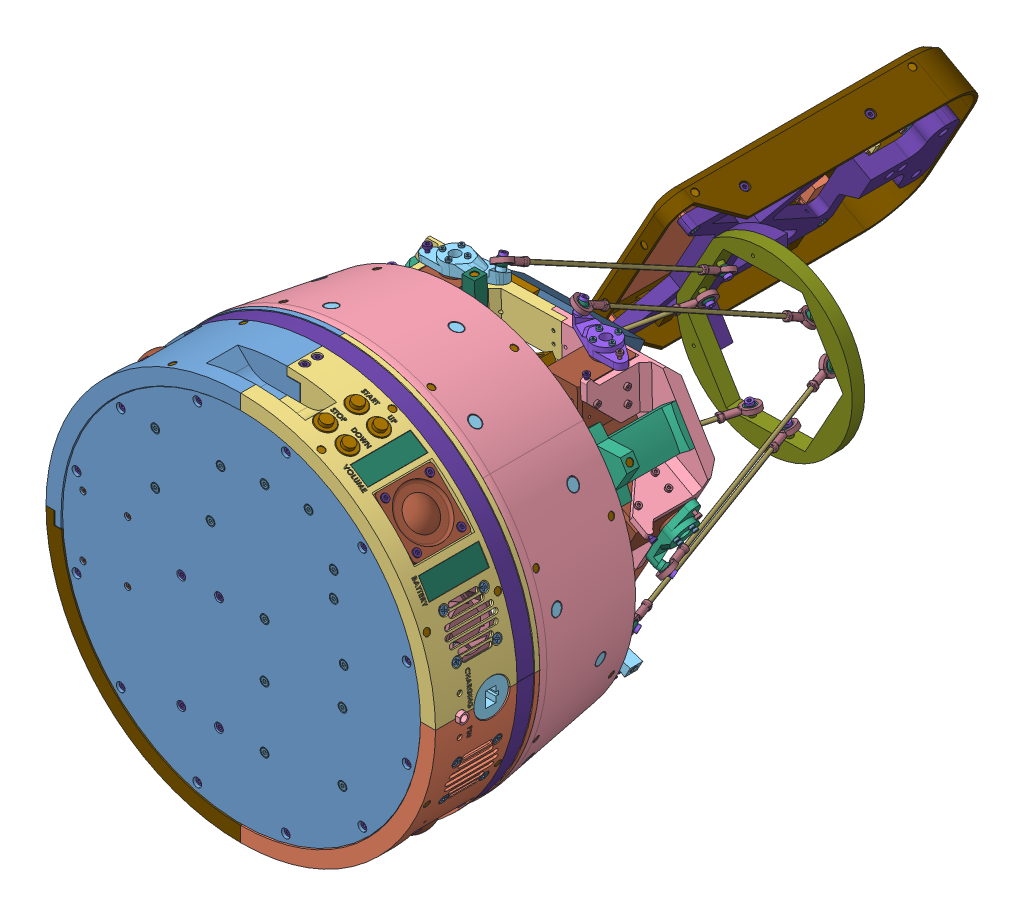
SolidWorks assembly robot xavier, configuration Défaut. Lengths in mm. (continued)
Components (placement in the parent): (continued)
- stewart-1: stewart [Défaut] at (-100.6475 26.8239 383.3519) x (-0.481912 -0.876219 0) z (0 0 1) size (270.43 245.67 405.82) (continued)
  - stewart bottom-1: stewart bottom [Défaut] at (51.9082 27.1683 257.1781) size (269.04 236.07 88.26) (flexible) (continued)
    - M2.5x8mm plastic-44: M2.5x8mm plastic [Défaut] at (-155.432 88.9962 153.3057) x (-0.891812 0 -0.452406) z (0 1 0) size (4.5 4.5 9.9)
    - M2.5x8mm plastic-45: M2.5x8mm plastic [Défaut] at (-0.6388 88.9962 153.514) x (0.993528 0 0.11359) z (0 1 0) size (4.5 4.5 9.9)
    - M2.5x8mm plastic-46: M2.5x8mm plastic [Défaut] at (43.8302 11.9975 156.9587) x (-0.496387 -0.859767 0.120004) z (0.866025 -0.5 0) size (4.5 4.5 9.9)
    - M3x8mm plastic-8: M3x8mm plastic [Défaut] at (-150.8412 50.5806 138.5562) x (0.25 0.433013 -0.866025) z (0.866025 -0.5 0) size (5.5 5.5 10.3)
    - M3x8mm plastic-9: M3x8mm plastic [Défaut] at (-164.3412 27.1979 138.5562) x (0.25 0.433013 -0.866025) z (0.866025 -0.5 0) size (5.5 5.5 10.3)
  - stewart rod-1: stewart rod [Défaut] at (34.7387 42.7785 243.5766) x (0.831609 0.550333 -0.074565) z (0.269993 -0.283304 0.920241) size (3 3 170)
  - stewart rod-2: stewart rod [Défaut] at (1.3025 -15.1346 243.6154) x (0.750903 0.658079 -0.055466) z (0.288475 -0.251293 0.923923) size (3 3 170)
  - stewart rod-3: stewart rod [Défaut] at (-69.2882 42.8434 243.2148) x (-0.526243 -0.723245 -0.447198) z (-0.37195 -0.277144 0.885914) size (3 3 170)
  - stewart rod-4: stewart rod [Défaut] at (-35.7774 -15.199 243.2264) x (0.751318 -0.64548 0.137392) z (-0.383348 -0.257403 0.887011) size (3 3 170)
  - stewart rod-5: stewart rod [Défaut] at (-50.6979 74.9201 243.922) x (-0.993577 0.094375 -0.062435) z (-0.031266 0.301309 0.953014) size (3 3 170)
  - stewart rod-6: stewart rod [Défaut] at (16.1837 74.9201 243.9023) x (0.359224 -0.882055 0.304856) z (-0.067343 0.301309 0.951145) size (3 3 170)
  - ball joint-1: ball joint [Défaut] at (86.3791 -15.0497 429.378) x (-0.641299 -0.765812 -0.047608) z (-0.269993 0.283304 -0.920241) size (14 8.06 27.54) (flexible)
    - ball joint body-1: ball joint body [Défaut] at (-2.323 -1.7007 27.3075) size (14 5.52 27.54)
    - ball joint liner-1: ball joint liner [Défaut] at (-2.323 -1.7007 20.7692) x (0.998229 0 -0.059488) z (0.059488 0 0.998229) size (9 3.5 9)
    - ball joint ball-1: ball joint ball [Défaut] at (-2.323 -1.7007 20.7692) x (-0.872539 0.157807 0.462355) z (-0.455394 0.079955 -0.886692) size (8 6 8)
  - ball joint-2: ball joint [Défaut] at (56.6193 -65.8542 430.4324) x (-0.789576 -0.608272 0.081087) z (-0.288475 0.251293 -0.923923) size (14 8.06 27.54) (flexible)
    - ball joint body-1: ball joint body [Défaut] at (-2.323 -1.7007 27.3075) size (14 5.52 27.54)
    - ball joint liner-1: ball joint liner [Défaut] at (-2.323 -1.7007 20.7692) x (0.94632 0 -0.323231) z (0.323231 0 0.94632) size (9 3.5 9)
    - ball joint ball-1: ball joint ball [Défaut] at (-2.323 -1.7007 20.7692) x (0.587551 -0.223397 -0.777738) z (0.725979 -0.278987 0.628586) size (8 6 8)
  - ball joint-3: ball joint [Défaut] at (-142.8187 -10.735 422.8134) x (-0.09653 0.960763 0.260032) z (0.37195 0.277144 -0.885914) size (14 8.06 27.54) (flexible)
    - ball joint body-1: ball joint body [Défaut] at (-2.323 -1.7007 27.3075) size (14 5.52 27.54)
    - ball joint liner-1: ball joint liner [Défaut] at (-2.323 -1.7007 20.7692) x (-0.616395 0 -0.787437) z (0.787437 0 -0.616395) size (9 3.5 9)
    - ball joint ball-1: ball joint ball [Défaut] at (-2.323 -1.7007 20.7692) x (0.165408 0.04529 -0.985185) z (0.919478 -0.368332 0.137444) size (8 6 8)
  - ball joint-4: ball joint [Défaut] at (-114.0751 -64.3814 422.0659) x (-0.810009 0.555134 -0.188975) z (0.383348 0.257403 -0.887011) size (14 8.06 27.54) (flexible)
    - ball joint body-1: ball joint body [Défaut] at (-2.323 -1.7007 27.3075) size (14 5.52 27.54)
    - ball joint liner-1: ball joint liner [Défaut] at (-2.323 -1.7007 20.7692) x (-0.982349 0 0.18706) z (-0.18706 0 -0.982349) size (9 3.5 9)
    - ball joint ball-1: ball joint ball [Défaut] at (-2.323 -1.7007 20.7692) x (0.172931 0.183122 -0.967761) z (0.917508 0.327341 0.225891) size (8 6 8)
  - ball joint-5: ball joint [Défaut] at (-0.0745 136.4534 434.9058) x (-0.957396 -0.287828 0.023394) z (0.067343 -0.301309 -0.951145) size (14 8.06 27.54) (flexible)
    - ball joint body-1: ball joint body [Défaut] at (-2.323 -1.7007 27.3075) size (14 5.52 27.54)
    - ball joint liner-1: ball joint liner [Défaut] at (-2.323 -1.7007 20.7692) x (-0.714828 0 0.6993) z (-0.6993 0 -0.714828) size (9 3.5 9)
    - ball joint ball-1: ball joint ball [Défaut] at (-2.323 -1.7007 20.7692) x (0.92076 0.200492 0.334671) z (-0.308893 -0.149333 0.9393) size (8 6 8)
  - ball joint-6: ball joint [Défaut] at (-58.7526 137.7306 435.0318) x (-0.960472 0.25482 -0.112076) z (0.031266 -0.301309 -0.953014) size (14 8.06 27.54) (flexible)
    - ball joint body-1: ball joint body [Défaut] at (-2.323 -1.7007 27.3075) size (14 5.52 27.54)
    - ball joint liner-1: ball joint liner [Défaut] at (-2.323 -1.7007 20.7692) x (-0.066426 0 0.997791) z (-0.997791 0 -0.066426) size (9 3.5 9)
    - ball joint ball-1: ball joint ball [Défaut] at (-2.323 -1.7007 20.7692) x (0.463327 -0.040267 -0.885272) z (0.854034 -0.246363 0.458183) size (8 6 8)
  - ball joint-7: ball joint [Défaut] at (28.9713 51.1868 213.8362) x (0.611438 -0.687853 -0.391154) z (0.269993 -0.283304 0.920241) size (14 8.06 27.54) (flexible)
    - ball joint body-1: ball joint body [Défaut] at (-2.323 -1.7007 27.3075) size (14 5.52 27.54)
    - ball joint liner-1: ball joint liner [Défaut] at (-2.323 -1.7007 20.7692) x (0.810022 0 0.5864) z (-0.5864 0 0.810022) size (9 3.5 9)
    - ball joint ball-1: ball joint ball [Défaut] at (-2.323 -1.7007 20.7692) x (-0.955028 0.27367 0.114134) z (-0.137201 -0.066622 -0.9883) size (8 6 8)
  - ball joint-8: ball joint [Défaut] at (21.1642 65.5917 214.2944) x (0.814856 -0.533495 0.226697) z (-0.067343 0.301309 0.951145) size (14 8.06 27.54) (flexible)
    - ball joint body-1: ball joint body [Défaut] at (-2.323 -1.7007 27.3075) size (14 5.52 27.54)
    - ball joint liner-1: ball joint liner [Défaut] at (-2.323 -1.7007 20.7692) x (0.990267 0 0.139182) z (-0.139182 0 0.990267) size (9 3.5 9)
    - ball joint ball-1: ball joint ball [Défaut] at (-2.323 -1.7007 20.7692) x (-0.414294 0.066271 -0.907727) z (0.825998 -0.391457 -0.405572) size (8 6 8)
  - ball joint-9: ball joint [Défaut] at (-59.2368 53.9166 215.5598) x (-0.006343 0.955126 0.296133) z (-0.37195 -0.277144 0.885914) size (14 8.06 27.54) (flexible)
    - ball joint body-1: ball joint body [Défaut] at (-2.323 -1.7007 27.3075) size (14 5.52 27.54)
    - ball joint liner-1: ball joint liner [Défaut] at (-2.323 -1.7007 20.7692) x (0.770033 0 -0.638005) z (0.638005 0 0.770033) size (9 3.5 9)
    - ball joint ball-1: ball joint ball [Défaut] at (-2.323 -1.7007 20.7692) x (-0.855754 0.383962 -0.346783) z (0.314359 -0.146489 -0.937934) size (8 6 8)
  - ball joint-10: ball joint [Défaut] at (-49.6158 68.2312 213.2212) x (0.619017 0.754451 -0.218223) z (-0.031266 0.301309 0.953014) size (14 8.06 27.54) (flexible)
    - ball joint body-1: ball joint body [Défaut] at (-2.323 -1.7007 27.3075) size (14 5.52 27.54)
    - ball joint liner-1: ball joint liner [Défaut] at (-2.323 -1.7007 20.7692) x (0.987977 0 -0.154599) z (0.154599 0 0.987977) size (9 3.5 9)
    - ball joint ball-1: ball joint ball [Défaut] at (-2.323 -1.7007 20.7692) x (-0.498287 -0.076288 -0.863649) z (0.860004 0.08291 -0.503507) size (8 6 8)
  - ball joint-11: ball joint [Défaut] at (-21.1891 -6.7985 216.6734) x (0.851424 -0.47068 0.231381) z (-0.383348 -0.257403 0.887011) size (14 8.06 27.54) (flexible)
    - ball joint body-1: ball joint body [Défaut] at (-2.323 -1.7007 27.3075) size (14 5.52 27.54)
    - ball joint liner-1: ball joint liner [Défaut] at (-2.323 -1.7007 20.7692) x (0.919675 0 -0.39268) z (0.39268 0 0.919675) size (9 3.5 9)
    - ball joint ball-1: ball joint ball [Défaut] at (-2.323 -1.7007 20.7692) x (-0.561763 -0.31173 -0.76632) z (0.717246 0.278105 -0.638918) size (8 6 8)
  - ball joint-12: ball joint [Défaut] at (-5.5073 -5.4469 214.4911) x (0.957486 0.077261 -0.27794) z (0.288475 -0.251293 0.923923) size (14 8.06 27.54) (flexible)
    - ball joint body-1: ball joint body [Défaut] at (-2.323 -1.7007 27.3075) size (14 5.52 27.54)
    - ball joint liner-1: ball joint liner [Défaut] at (-2.323 -1.7007 20.7692) x (0.90176 0 0.432237) z (-0.432237 0 0.90176) size (9 3.5 9)
    - ball joint ball-1: ball joint ball [Défaut] at (-2.323 -1.7007 20.7692) x (-0.462126 -0.039425 -0.885938) z (0.886636 -0.040577 -0.460684) size (8 6 8)
  - stewart top-2: stewart top [Défaut] at (-16.7375 35.0075 227.064) x (-1 0 0) z (0 0 1) size (140 133 13.97)
  - head-1: head [Défaut] at (6.4848 -0.42 401.5084) x (1 0 0) z (0 0 -1) size (144.45 66.3 235)
    - head-1: head [Défaut] at (-23.2223 -35.4275 174.4445) size (127.79 46.8 223.89)
    - head cable protector-1: head cable protector [Défaut] at (-23.4875 51.0725 312.5758) x (1 0 0) z (0 -1 0) size (144.45 235 38)
    - Intel RealSense D435i-1: Intel RealSense D435i [Défaut] at (-23.2223 33.5725 341.3334) x (1 0 0) z (0 -1 0) size (90.36 24.95 25.31)
    - screen-1: screen [Défaut] at (-28.4523 45.5725 212.8445) x (0 0 1) z (0 1 0) size (166.25 124 16.51)
    - wide angle camera-1: wide angle camera [Défaut] at (-56.3573 32.5725 309.1237) x (1 0 0) z (0 -1 0) size (32 32 30.75)
    - M2.5x5mm plastic-2: M2.5x5mm plastic [Défaut] at (-70.1476 36.3225 295.3334) x (-1 0 0) z (0 -1 0) size (4.5 4.5 6.9)
    - M2.5x5mm plastic-3: M2.5x5mm plastic [Défaut] at (-42.567 36.3225 322.914) x (1 0 0) z (0 -1 0) size (4.5 4.5 6.9)
    - M2.5x5mm plastic-4: M2.5x5mm plastic [Défaut] at (-70.1476 36.3225 322.914) x (1 0 0) z (0 -1 0) size (4.5 4.5 6.9)
    - M3x12mm plastic-1: M3x12mm plastic [Défaut] at (-25.7223 35.0725 318.3334) x (1 0 0) z (0 -1 0) size (5.5 5.5 14.3)
    - M3x12mm plastic-2: M3x12mm plastic [Défaut] at (-25.7223 35.0725 308.3334) x (1 0 0) z (0 -1 0) size (5.5 5.5 14.3)
    - M3x10mm socket-1: M3x10mm socket [Défaut] at (-45.7223 30.8225 341.3334) x (1 0 0) z (0 -1 0) size (5.5 5.5 13)
    - M3x10mm socket-2: M3x10mm socket [Défaut] at (-0.7223 30.8225 341.3334) x (1 0 0) z (0 -1 0) size (5.5 5.5 13)
    - M3x5mm socket-1: M3x5mm socket [Défaut] at (-85.9923 42.2925 291.3445) x (1 0 0) z (0 1 0) size (5.5 5.5 8)
    - M3x5mm socket-2: M3x5mm socket [Défaut] at (29.0877 42.2925 291.3445) x (1 0 0) z (0 1 0) size (5.5 5.5 8)
    - M3x5mm socket-3: M3x5mm socket [Défaut] at (-85.9923 42.2925 134.4445) x (1 0 0) z (0 1 0) size (5.5 5.5 8)
    - M3x5mm socket-4: M3x5mm socket [Défaut] at (29.0877 42.2925 134.4445) x (1 0 0) z (0 1 0) size (5.5 5.5 8)
    - M3x10mm socket-3: M3x10mm socket [Défaut] at (-85.9923 40.5725 291.3445) x (1 0 0) z (0 -1 0) size (5.5 5.5 13)
    - M3x10mm socket-4: M3x10mm socket [Défaut] at (-85.9923 40.5725 134.4445) x (1 0 0) z (0 -1 0) size (5.5 5.5 13)
    - M3x10mm socket-5: M3x10mm socket [Défaut] at (29.0877 40.5725 134.4445) x (1 0 0) z (0 -1 0) size (5.5 5.5 13)
    - M3x10mm socket-6: M3x10mm socket [Défaut] at (29.0877 40.5725 291.3445) x (1 0 0) z (0 -1 0) size (5.5 5.5 13)
    - M2.5x5mm plastic-1: M2.5x5mm plastic [Défaut] at (-42.567 36.3225 295.3334) x (-1 0 0) z (0 -1 0) size (4.5 4.5 6.9)
    - magnet 5x1.6-1: magnet 5x1.6 [Défaut] at (48.5977 44.0725 317.3334) x (0 0 1) z (-1 0 0) size (5 5 1.6)
    - magnet 5x1.6-2: magnet 5x1.6 [Défaut] at (7.9977 44.0725 356.3334) size (5 5 1.6)
    - magnet 5x1.6-3: magnet 5x1.6 [Défaut] at (-54.4523 44.0725 356.3334) size (5 5 1.6)
    - magnet 5x1.6-4: magnet 5x1.6 [Défaut] at (-95.0523 44.0725 317.3334) x (0 0 -1) z (1 0 0) size (5 5 1.6)
    - magnet 5x1.6-5: magnet 5x1.6 [Défaut] at (-93.4523 44.0725 144.3334) x (0 0 1) z (-1 0 0) size (5 5 1.6)
    - magnet 5x1.6-6: magnet 5x1.6 [Défaut] at (46.9977 44.0725 144.3334) x (0 0 -1) z (1 0 0) size (5 5 1.6)
    - M3x8mm plastic-1: M3x8mm plastic [Défaut] at (-84.4523 32.5725 273.9445) x (0 0.924225 0.381849) z (-1 0 0) size (5.5 5.5 10.3)
    - M3x8mm plastic-2: M3x8mm plastic [Défaut] at (-84.4523 32.5725 173.9445) x (0 0.924225 0.381849) z (-1 0 0) size (5.5 5.5 10.3)
    - M3x8mm plastic-3: M3x8mm plastic [Défaut] at (27.5477 32.5725 173.9445) x (0 0 -1) z (1 0 0) size (5.5 5.5 10.3)
    - M3x8mm plastic-4: M3x8mm plastic [Défaut] at (27.5477 32.5725 273.9445) x (0 0 -1) z (1 0 0) size (5.5 5.5 10.3)
    - magnet 5x1.6-7: magnet 5x1.6 [Défaut] at (7.9977 44.0725 123.7334) size (5 5 1.6)
    - magnet 5x1.6-8: magnet 5x1.6 [Défaut] at (-54.4523 44.0725 123.7334) size (5 5 1.6)
  - M3x12mm plastic-1: M3x12mm plastic [Défaut] at (76.1049 -4.4795 413.0978) x (0.534054 0.339834 0.774144) z (0.819766 -0.432128 -0.375831) size (5.5 5.5 14.3)
  - M3x12mm plastic-2: M3x12mm plastic [Défaut] at (46.2864 -56.1267 413.8081) x (-0.606362 -0.716834 -0.3442) z (0.788544 -0.486207 -0.376565) size (5.5 5.5 14.3)
  - M3x12mm plastic-3: M3x12mm plastic [Défaut] at (-98.2887 -56.6028 406.6005) x (-0.589644 0.3009 0.749519) z (-0.744184 -0.56304 -0.35941) size (5.5 5.5 14.3)
  - M3x12mm plastic-4: M3x12mm plastic [Défaut] at (-128.6903 -3.9456 406.3833) x (-0.469672 0.293478 0.832634) z (-0.861016 -0.360681 -0.358553) size (5.5 5.5 14.3)
  - M3x12mm plastic-5: M3x12mm plastic [Défaut] at (4.3737 120.984 419.0003) x (-0.283643 -0.370525 -0.884453) z (-0.038662 0.926002 -0.375533) size (5.5 5.5 14.3)
  - M3x12mm plastic-6: M3x12mm plastic [Défaut] at (-56.731 120.984 419.3529) x (-0.967301 -0.055183 -0.247555) z (0.043155 0.926002 -0.375043) size (5.5 5.5 14.3)
  - M3x12mm plastic-7: M3x12mm plastic [Défaut] at (39.5173 50.1657 232.0076) x (0.451147 -0.868576 -0.205042) z (-0.847101 -0.489074 0.207912) size (5.5 5.5 14.3)
  - M3x12mm plastic-8: M3x12mm plastic [Défaut] at (24.5173 76.1465 232.0076) x (0.099546 0.238276 0.966082) z (-0.847101 -0.489074 0.207912) size (5.5 5.5 14.3)
  - M3x12mm plastic-9: M3x12mm plastic [Défaut] at (-72.9924 50.1657 232.0076) x (0.405934 0.342984 -0.847101) z (0.847101 -0.489074 0.207912) size (5.5 5.5 14.3)
  - M3x12mm plastic-10: M3x12mm plastic [Défaut] at (-57.9924 76.1465 232.0076) x (0.405934 0.342984 -0.847101) z (0.847101 -0.489074 0.207912) size (5.5 5.5 14.3)
  - M3x12mm plastic-11: M3x12mm plastic [Défaut] at (-31.7375 -21.2898 232.0076) x (0.89063 -0.094544 0.444792) z (0 0.978148 0.207912) size (5.5 5.5 14.3)
  - M3x12mm plastic-12: M3x12mm plastic [Défaut] at (-1.7375 -21.2898 232.0076) x (1 0 0) z (0 0.978148 0.207912) size (5.5 5.5 14.3)
  - M3x12mm plastic-13: M3x12mm plastic [Défaut] at (32.0884 -2.1725 233.064) x (-0.923728 -0.383049 0) z (0 0 -1) size (5.5 5.5 14.3)
  - M3x12mm plastic-14: M3x12mm plastic [Défaut] at (-65.5634 -2.1725 233.064) x (-1 0 0) z (0 0 -1) size (5.5 5.5 14.3)
  - M3x12mm plastic-15: M3x12mm plastic [Défaut] at (3.2625 -21.9925 232.064) x (1 0 0) z (0 -1 0) size (5.5 5.5 14.3)
  - M3x12mm plastic-16: M3x12mm plastic [Défaut] at (-36.7375 -21.9925 232.064) x (1 0 0) z (0 -1 0) size (5.5 5.5 14.3)
- M3x12mm plastic-1: M3x12mm plastic [Défaut] at (-70.4088 173.5241 871.5862) x (-0.924031 0.382318 0) z (0 0 -1) size (5.5 5.5 14.3)
- M3x12mm plastic-16: M3x12mm plastic [Défaut] at (-19.3206 163.362 871.5862) x (-0.707387 0.706827 0) z (0 0 -1) size (5.5 5.5 14.3)
- M3x12mm plastic-15: M3x12mm plastic [Défaut] at (23.9899 134.4228 871.5862) x (-0.383049 0.923728 0) z (0 0 -1) size (5.5 5.5 14.3)
- M3x12mm plastic-14: M3x12mm plastic [Défaut] at (52.9291 91.1123 871.5862) x (-0.000396 1 0) z (0 0 -1) size (5.5 5.5 14.3)
- M3x12mm plastic-13: M3x12mm plastic [Défaut] at (63.0912 40.0241 871.5862) x (0.382318 0.924031 0) z (0 0 -1) size (5.5 5.5 14.3)
- M3x12mm plastic-12: M3x12mm plastic [Défaut] at (52.9291 -11.0642 871.5862) x (0.706827 0.707387 0) z (0 0 -1) size (5.5 5.5 14.3)
- M3x12mm plastic-11: M3x12mm plastic [Défaut] at (23.9899 -54.3747 871.5862) x (0.923728 0.383049 0) z (0 0 -1) size (5.5 5.5 14.3)
- M3x12mm plastic-10: M3x12mm plastic [Défaut] at (-19.3206 -83.3139 871.5862) x (1 0.000396 0) z (0 0 -1) size (5.5 5.5 14.3)
- M3x12mm plastic-9: M3x12mm plastic [Défaut] at (-70.4088 -93.4759 871.5862) x (0.924031 -0.382318 0) z (0 0 -1) size (5.5 5.5 14.3)
- M3x12mm plastic-8: M3x12mm plastic [Défaut] at (-121.4971 -83.3139 871.5862) x (0.707387 -0.706827 0) z (0 0 -1) size (5.5 5.5 14.3)
- M3x12mm plastic-7: M3x12mm plastic [Défaut] at (-164.8076 -54.3747 871.5862) x (0.383049 -0.923728 0) z (0 0 -1) size (5.5 5.5 14.3)
- M3x12mm plastic-6: M3x12mm plastic [Défaut] at (-193.7467 -11.0642 871.5862) x (0.000396 -1 0) z (0 0 -1) size (5.5 5.5 14.3)
- M3x12mm plastic-5: M3x12mm plastic [Défaut] at (-203.9088 40.0241 871.5862) x (-0.382318 -0.924031 0) z (0 0 -1) size (5.5 5.5 14.3)
- M3x12mm plastic-4: M3x12mm plastic [Défaut] at (-193.7467 91.1123 871.5862) x (-0.706827 -0.707387 0) z (0 0 -1) size (5.5 5.5 14.3)
- M3x12mm plastic-3: M3x12mm plastic [Défaut] at (-164.8076 134.4228 871.5862) x (-0.923728 -0.383049 0) z (0 0 -1) size (5.5 5.5 14.3)
- M3x12mm plastic-2: M3x12mm plastic [Défaut] at (-121.4971 163.362 871.5862) x (-1 -0.000396 0) z (0 0 -1) size (5.5 5.5 14.3)
- M3x12mm plastic-17: M3x12mm plastic [Défaut] at (-176.1027 89.5952 790.5862) x (-0.997337 0.072935 0) z (0 0 -1) size (5.5 5.5 14.3)
- M3x12mm plastic-18: M3x12mm plastic [Défaut] at (-168.874 102.7385 790.5862) x (-0.876347 0.48168 0) z (0 0 -1) size (5.5 5.5 14.3)
- M3x12mm plastic-19: M3x12mm plastic [Défaut] at (-75.4902 -76.6037 790.5862) x (-0.998479 0.055124 0) z (0 0 -1) size (5.5 5.5 14.3)
- M3x12mm plastic-20: M3x12mm plastic [Défaut] at (-60.4935 -76.2923 790.5862) x (-0.995663 0.093037 0) z (0 0 -1) size (5.5 5.5 14.3)
- M3x12mm plastic-21: M3x12mm plastic [Défaut] at (33.1328 93.9402 790.5862) x (-0.863886 0.503687 0) z (0 0 -1) size (5.5 5.5 14.3)
- M3x12mm plastic-22: M3x12mm plastic [Défaut] at (25.3647 106.772 790.5862) x (-0.865278 0.501292 0) z (0 0 -1) size (5.5 5.5 14.3)
Mates (geometry in assembly coordinates):
- Coïncidente1: coincident anti-aligned: plane of base-1/base mic-1/base mic-3 through (-162.6654 132.2807 865.5862) normal (0 0 -1); plane of torso bottom xavier-1/base gear-1/base gear 2-1 through (-178.4088 40.0241 865.5862) normal (0 0 1)
- Coaxiale3: concentric anti-aligned: cylinder of torso bottom xavier-1/base gear-1/base gear 3-1 through (-70.4088 173.5241 865.5872) axis (0 0 -1) radius 1.75; cylinder of M3x12mm plastic-1 through (-70.4088 173.5241 859.5862) axis (0 0 1) radius 1.5
- Coïncidente2: coincident aligned: plane of torso bottom xavier-1/base gear-1/base gear 3-1 through (-70.4088 173.5241 859.5862) normal (0 0 -1); circle of M3x12mm plastic-1
- Coaxiale4: concentric aligned: cylinder of base-1/base mic-1/base mic-1 through (63.0912 40.0241 945.5872) axis (0 0 -1) radius 1.25; cylinder of torso bottom xavier-1/base gear-1/base gear 4-1 through (63.0912 40.0241 865.5872) axis (0 0 -1) radius 1.75
- Coaxiale5: concentric aligned: cylinder of base-1/base mic-1/base mic-1 through (52.9291 91.1123 945.5872) axis (0 0 -1) radius 1.25; cylinder of torso bottom xavier-1/base gear-1/base gear 3-1 through (52.9291 91.1123 865.5872) axis (0 0 -1) radius 1.75
- Coïncidente3: coincident anti-aligned: plane of torso bottom xavier-1/stewart bracket-2 through (-70.4088 40.0241 784.5862) normal (0 0 -1); plane of stewart-1/stewart bottom-1/stewart bottom 2-1 through (-70.4105 40.025 784.5862) normal (0 0 1)
- Coaxiale6: concentric aligned: cylinder of torso bottom xavier-1/stewart bracket-2 through (-176.1027 89.5952 794.5862) axis (0 0 -1) radius 1.25; cylinder of stewart-1/stewart bottom-1/stewart bottom 2-1 through (-176.1027 89.5952 804.5872) axis (0 0 -1) radius 1.75
- Coaxiale7: concentric aligned: cylinder of torso bottom xavier-1/stewart bracket-2 through (-168.874 102.7385 794.5862) axis (0 0 -1) radius 1.25; cylinder of stewart-1/stewart bottom-1/stewart bottom 2-1 through (-168.874 102.7385 804.5872) axis (0 0 -1) radius 1.75
- Coaxiale8: concentric anti-aligned: cylinder of stewart-1/stewart bottom-1/stewart bottom 1-1 through (-60.4935 -76.2923 804.5872) axis (0 0 -1) radius 1.75; cylinder of M3x12mm plastic-20 through (-60.4935 -76.2923 778.5862) axis (0 0 1) radius 1.5
- Coïncidente4: coincident aligned: plane of stewart-1/stewart bottom-1/stewart bottom 1-1 through (-60.4935 -76.2923 778.5862) normal (0 0 -1); circle of M3x12mm plastic-20
- Coaxiale9: concentric anti-aligned: cylinder of stewart-1/stewart bottom-1/stewart bottom 1-1 through (-75.4902 -76.6037 804.5872) axis (0 0 -1) radius 1.75; cylinder of M3x12mm plastic-19 through (-75.4902 -76.6037 778.5862) axis (0 0 1) radius 1.5
- Coïncidente5: coincident aligned: plane of stewart-1/stewart bottom-1/stewart bottom 1-1 through (-75.4902 -76.6037 778.5862) normal (0 0 -1); circle of M3x12mm plastic-19
- Coaxiale10: concentric anti-aligned: cylinder of stewart-1/stewart bottom-1/stewart bottom 2-1 through (-176.1027 89.5952 804.5872) axis (0 0 -1) radius 1.75; cylinder of M3x12mm plastic-17 through (-176.1027 89.5952 778.5862) axis (0 0 1) radius 1.5
- Coïncidente6: coincident aligned: plane of stewart-1/stewart bottom-1/stewart bottom 2-1 through (-176.1027 89.5952 778.5862) normal (0 0 -1); circle of M3x12mm plastic-17
- Coaxiale11: concentric anti-aligned: cylinder of stewart-1/stewart bottom-1/stewart bottom 2-1 through (-168.874 102.7385 804.5872) axis (0 0 -1) radius 1.75; cylinder of M3x12mm plastic-18 through (-168.874 102.7385 778.5862) axis (0 0 1) radius 1.5
- Coïncidente7: coincident aligned: plane of stewart-1/stewart bottom-1/stewart bottom 2-1 through (-168.874 102.7385 778.5862) normal (0 0 -1); circle of M3x12mm plastic-18
- Coaxiale12: concentric anti-aligned: cylinder of stewart-1/stewart bottom-1/stewart bottom 3-1 through (25.3647 106.772 804.5872) axis (0 0 -1) radius 1.75; cylinder of M3x12mm plastic-22 through (25.3647 106.772 778.5862) axis (0 0 1) radius 1.5
- Coïncidente8: coincident aligned: plane of stewart-1/stewart bottom-1/stewart bottom 3-1 through (25.3647 106.772 778.5862) normal (0 0 -1); circle of M3x12mm plastic-22
- Coaxiale13: concentric anti-aligned: cylinder of stewart-1/stewart bottom-1/stewart bottom 3-1 through (33.1328 93.9402 804.5872) axis (0 0 -1) radius 1.75; cylinder of M3x12mm plastic-21 through (33.1328 93.9402 778.5862) axis (0 0 1) radius 1.5
- Coïncidente9: coincident aligned: plane of stewart-1/stewart bottom-1/stewart bottom 3-1 through (33.1328 93.9402 778.5862) normal (0 0 -1); circle of M3x12mm plastic-21
